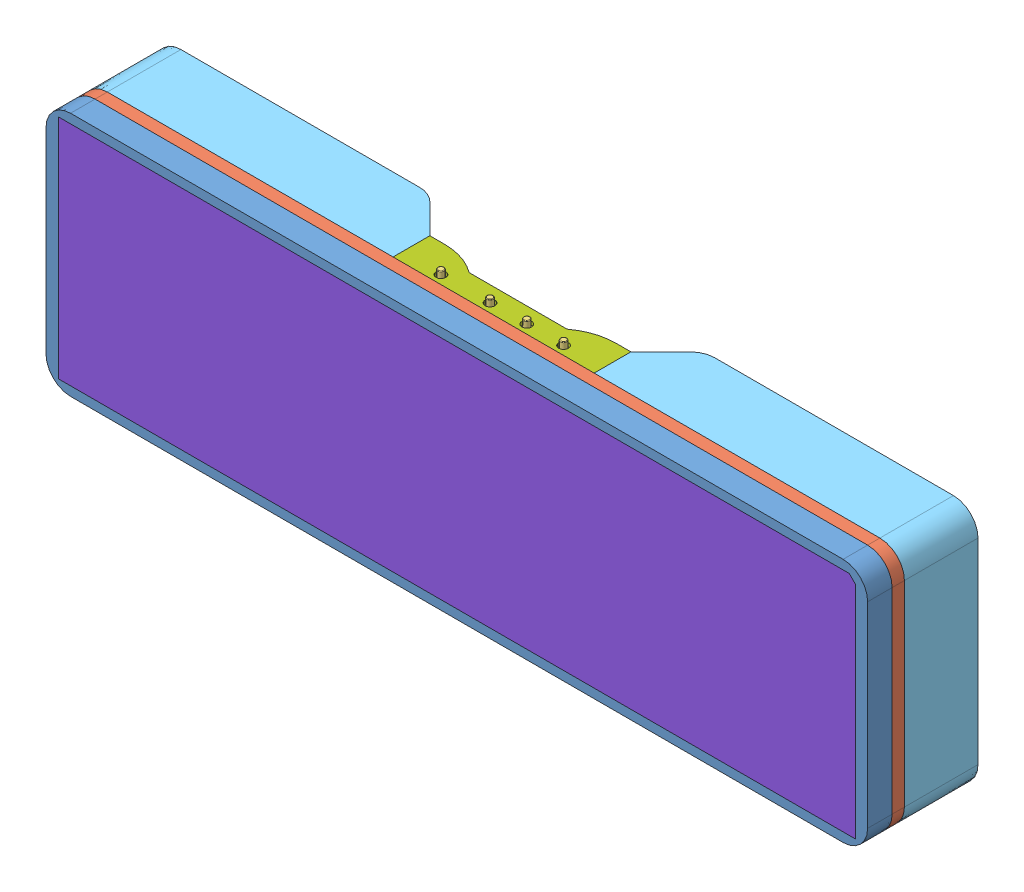
SolidWorks assembly bluetooth_clock_assembly, configuration Default. Lengths in mm.
Overall size (335 102.08 45).
13 component instances, 8 part files, 16 mates.
Components (placement in the parent):
- front_panel-1: front_panel [Default] at origin size (335 100 10)
- mid_panel-1: mid_panel [Default] at (0 0 -10) size (335 100 5)
- bluetooth_clock-1: bluetooth_clock [Default] at (40 -3 -15.4115) x (-1 0 0) z (0 0 -1) size (81.03 55.08 13.6)
- neopixel_8x32_matrix-1: neopixel_8x32_matrix [Default] at (-121.9619 16.53 -1.0098) size (266 65 3.1)
  - Neopixel Led-1: Neopixel Led [Predeterminado] at (54.8048 13.4445 -8.9902) x (-1 0 0) z (0 1 0) size (65 3.1 65)
  - Neopixel Led-5: Neopixel Led [Predeterminado] at (121.8048 13.4445 -8.9902) x (-1 0 0) z (0 1 0) size (65 3.1 65)
  - Neopixel Led-6: Neopixel Led [Predeterminado] at (188.8048 13.4445 -8.9902) x (-1 0 0) z (0 1 0) size (65 3.1 65)
  - Neopixel Led-7: Neopixel Led [Predeterminado] at (255.8048 13.4445 -8.9902) x (-1 0 0) z (0 1 0) size (65 3.1 65)
- back_panel-1: back_panel [Default] at (0 0 -45) x (-1 0 0) z (0 0 -1) size (335 100 30)
- 50mm_3W_spkr-2: 50mm_3W_spkr [Default] at (-122.5 0 -37.1) size (52.5 52.5 22.91)
- 50mm_3W_spkr-3: 50mm_3W_spkr [Default] at (122.5 0 -37.1) size (52.5 52.5 22.91)
- back_cover-1: back_cover [Default] at (0 -2 -22.5) x (-1 0 0) z (0 0 -1) size (82 52 15)
- plexiglass_black-1: plexiglass_black [Default] at (0 0 -2) size (325 92.5 2)
Mates (geometry in assembly coordinates):
- Coincident1: coincident aligned: line of front_panel-1 through (167.5 -40 -10) axis (0 1 0); line of mid_panel-1 through (167.5 -40 -10) axis (0 1 0)
- Coincident2: coincident aligned: line of front_panel-1 through (157.5 50 -10) axis (-1 0 0); line of mid_panel-1 through (157.5 50 -10) axis (-1 0 0)
- Coincident4: coincident anti-aligned: circle of mid_panel-1; circle of bluetooth_clock-1
- Coincident5: coincident anti-aligned: plane of mid_panel-1 through (0 0 -10) normal (0 0 1); plane of neopixel_8x32_matrix-1/Neopixel Led-6 through (66.8428 29.9745 -10) normal (0 0 -1)
- Coincident8: coincident anti-aligned: plane of mid_panel-1 through (0 0 -15) normal (0 0 -1); plane of back_panel-1 through (0 0 -15) normal (0 0 1)
- Coincident9: coincident aligned: line of mid_panel-1 through (167.5 -40 -15) axis (0 1 0); line of back_panel-1 through (167.5 -40 -15) axis (0 1 0)
- Coincident10: coincident aligned: line of mid_panel-1 through (157.5 50 -15) axis (-1 0 0); line of back_panel-1 through (157.5 50 -15) axis (-1 0 0)
- Coincident11: coincident anti-aligned: plane of back_panel-1 through (41 -2 -40) normal (-1 0 0); plane of back_cover-1 through (41 50 -30) normal (1 0 0)
- Coincident12: coincident aligned: line of back_panel-1 through (41 50 -30) axis (0 -1 0); line of back_cover-1 through (41 50 -30) axis (0 -1 0)
- Coincident13: coincident anti-aligned: line of back_panel-1 through (-41 50 -15) axis (0 0 -1); line of back_cover-1 through (-41 50 -30) axis (0 0 1)
- Coincident14: coincident aligned: line of front_panel-1 through (87.5 -162.5 43.75) axis (0 0 -1); line of plexiglass_black-1 through (92.5 -162.5 46.25) axis (0 0 -1)
- Coincident15: coincident anti-aligned: plane of front_panel-1 through (-162.5 46.25 -10) normal (0 -1 0); plane of plexiglass_black-1 through (-162.5 46.25 0) normal (0 1 0)
- Concentric2: concentric anti-aligned: cylinder of mid_panel-1 through (-122.5 0 -15) axis (0 0 1) radius 25.5; cylinder of 50mm_3W_spkr-2 through (-122.5 0 -29.6415) axis (0 0 -1) radius 25
- Concentric3: concentric anti-aligned: cylinder of mid_panel-1 through (122.5 0 -15) axis (0 0 1) radius 25.5; cylinder of 50mm_3W_spkr-3 through (122.5 0 -29.6415) axis (0 0 -1) radius 25
- Coincident16: coincident anti-aligned: plane of mid_panel-1 through (0 0 -15) normal (0 0 -1); plane of 50mm_3W_spkr-2 through (-156.65 0 -15) normal (0 0 1)
- Coincident17: coincident anti-aligned: plane of mid_panel-1 through (0 0 -15) normal (0 0 -1); plane of 50mm_3W_spkr-3 through (88.35 0 -15) normal (0 0 1)
